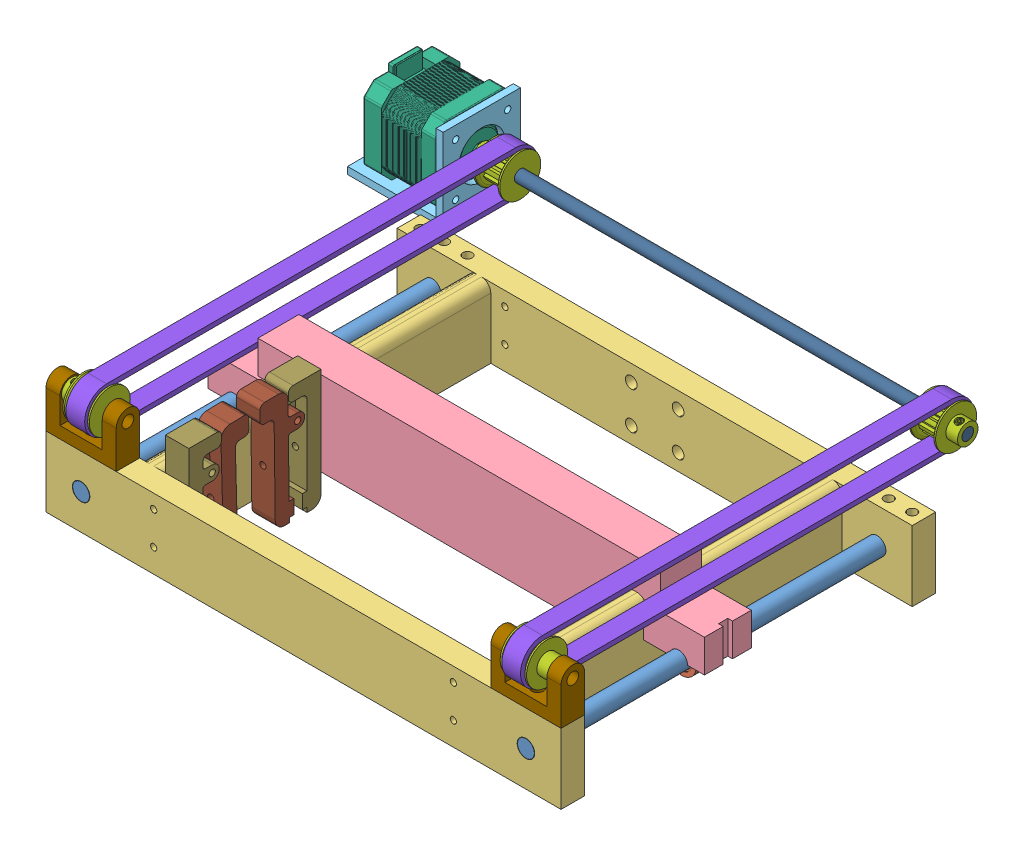
SolidWorks assembly Gantry Assembly Vertical Pulleys, configuration Default. Lengths in mm.
Overall size (322.83 91.67 256.35).
24 component instances, 12 part files, 42 mates.
Components (placement in the parent):
- 1555T132_Linear Motion Shaft-1: 1555T132_Linear Motion Shaft [1555T132] at (256.3952 90.1087 151.9483) x (0.714788 0.699342 0) z (0 0 1) size (9.53 9.53 203.2)
- 6630K12_Self-Aligning Linear Ball Bearing-1: 6630K12_Self-Aligning Linear Ball Bearing [6630K12] at (256.3952 90.1087 157.9768) size (15.88 15.88 22.23)
- Frame-1: Frame [Default] at (135.7452 70.9617 151.9483) x (0 0 -1) z (1 0 0) size (203.2 38.1 279.4)
- Singular Gantry-1: Singular Gantry [Default] at (135.7452 107.8887 157.9768) size (269.24 45.72 25.4)
- 1555T132_Linear Motion Shaft-2: 1555T132_Linear Motion Shaft [1555T132] at (15.0952 90.1087 151.9483) x (-0.570511 -0.82129 0) z (0 0 -1) size (9.53 9.53 203.2)
- 6630K12_Self-Aligning Linear Ball Bearing-2: 6630K12_Self-Aligning Linear Ball Bearing [6630K12] at (15.0952 90.1087 157.9768) x (0.996009 -0.089256 0) z (0 0 1) size (15.88 15.88 22.23)
- Mount and Motor-1: Mount and Motor [Default] at (-234.8386 169.217 17.6112) x (0 0 -1) z (1 0 0) size (42.51 50.31 70.26)
  - Mount (not Blake)-1: Mount (not Blake) [Default] at (-7.9724 -40.1303 235.4559) x (0 0 1) z (0 1 0) size (51.82 41.92 45.73)
  - Stepper Motor-1: Stepper Motor [Default] at (-7.6774 -39.8353 216.7059) size (42.5 46.5 61.75)
- 6495K744_Timing Belt Pulley-9: 6495K744_Timing Belt Pulley [6495K744] at (14.7396 129.3817 25.2886) x (0 -0.489559 0.87197) z (-1 0 0) size (22.23 22.23 20.62)
- Linear Rod Belt-1: Linear Rod Belt [Default] at (259.0495 129.3817 136.2434) x (0 0 -1) z (0 1 0) size (245.79 10.16 23.88)
- Linear Rod Belt-2: Linear Rod Belt [Default] at (12.4409 129.3817 136.2434) x (0 0 -1) z (0 -1 0) size (245.79 10.16 23.88)
- 6495K744_Timing Belt Pulley-10: 6495K744_Timing Belt Pulley [6495K744] at (13.9776 129.3817 247.1983) x (0 0.986803 0.161926) z (-1 0 0) size (22.23 22.23 20.62)
- Sideways Pulley Holder-1: Sideways Pulley Holder [Default] at (-3.9548 109.0617 247.1983) size (38.1 26.67 12.7)
- Sideways Pulley Holder-2: Sideways Pulley Holder [Default] at (237.3452 109.0617 247.1983) size (38.1 26.67 12.7)
- 6495K744_Timing Belt Pulley-11: 6495K744_Timing Belt Pulley [6495K744] at (257.5128 129.3817 247.1983) x (0 -0.977894 -0.209101) z (1 0 0) size (22.23 22.23 20.62)
- 6495K744_Timing Belt Pulley-12: 6495K744_Timing Belt Pulley [6495K744] at (257.5128 129.3817 25.2886) x (0 0.264564 -0.964368) z (1 0 0) size (22.23 22.23 20.62)
- Sideways Pulley Long Axle-1: Sideways Pulley Long Axle [Default] at (267.8252 129.3817 25.2886) x (0 -0.963895 0.266284) z (0 -0.266284 -0.963895) size (6.35 254 6.35)
- Clip Assembly-3: Clip Assembly [Default] at (102.1447 55.2873 173.3888) x (0 0.02134 0.999772) z (-1 0 0) size (34.59 64.43 12.7) (flexible)
  - Added Clip Piece-1: Added Clip Piece [Default] at (17.9829 40.6841 41.3294) x (0.999416 -0.034157 0) z (0 0 1) size (24.13 63.5 12.7)
  - Attatched Clip Piece-1: Attatched Clip Piece [Default] at (0.3891 41.1725 54.0294) x (-0.999772 0.02134 0) z (0 0 -1) size (17.78 63.5 12.7)
- Clip Assembly-5: Clip Assembly [Default] at (6.7858 53.9203 236.5487) x (0 0.02134 -0.999772) z (1 0 0) size (34.27 63.86 12.7) (flexible)
  - Added Clip Piece-1: Added Clip Piece [Default] at (18.5505 41.0342 41.3294) x (0.999981 0.006111 0) z (0 0 1) size (24.13 63.5 12.7)
  - Attatched Clip Piece-1: Attatched Clip Piece [Default] at (0.3891 41.1725 54.0294) x (-0.999772 0.02134 0) z (0 0 -1) size (17.78 63.5 12.7)
Mates (geometry in assembly coordinates):
- Concentric1: concentric anti-aligned: cylinder of 6630K12_Self-Aligning Linear Ball Bearing-1 through (256.3952 90.1087 169.0893) axis (0 0 -1) radius 7.9375; cylinder of Singular Gantry-1 through (256.3952 90.1087 146.8643) axis (0 0 1) radius 7.9375
- Coincident1: coincident anti-aligned: plane of 6630K12_Self-Aligning Linear Ball Bearing-1 through (256.3952 90.1087 146.8643) normal (0 0 -1); plane of Singular Gantry-1 through (15.0952 90.1087 146.8643) normal (0 0 1)
- Concentric2: concentric aligned: cylinder of 1555T132_Linear Motion Shaft-1 through (256.3952 90.1087 253.5483) axis (0 0 -1) radius 4.7625; cylinder of 6630K12_Self-Aligning Linear Ball Bearing-1 through (256.3952 90.1087 169.0893) axis (0 0 -1) radius 4.8895
- Concentric3: concentric anti-aligned: cylinder of 1555T132_Linear Motion Shaft-1 through (256.3952 90.1087 253.5483) axis (0 0 -1) radius 4.7625; cylinder of Frame-1 through (256.3952 90.1087 -189.6817) axis (0 0 1) radius 4.7625
- Concentric4: concentric aligned: cylinder of Frame-1 through (15.0952 90.1087 -189.6817) axis (0 0 1) radius 4.7625; cylinder of 1555T132_Linear Motion Shaft-2 through (15.0952 90.1087 50.3483) axis (0 0 1) radius 4.7625
- Parallel1: parallel aligned: plane of Frame-1 through (135.7452 109.0617 151.9483) normal (0 1 0); plane of Singular Gantry-1 through (26.5252 125.6687 146.8643) normal (0 1 0)
- Concentric5: concentric anti-aligned: cylinder of Singular Gantry-1 through (15.0952 90.1087 146.8643) axis (0 0 1) radius 7.9375; cylinder of 6630K12_Self-Aligning Linear Ball Bearing-2 through (15.0952 90.1087 169.0893) axis (0 0 -1) radius 7.9375
- Coincident2: coincident anti-aligned: plane of Singular Gantry-1 through (15.0952 90.1087 146.8643) normal (0 0 1); plane of 6630K12_Self-Aligning Linear Ball Bearing-2 through (15.0952 90.1087 146.8643) normal (0 0 -1)
- Concentric6: concentric anti-aligned: cylinder of 1555T132_Linear Motion Shaft-2 through (15.0952 90.1087 50.3483) axis (0 0 1) radius 4.7625; cylinder of 6630K12_Self-Aligning Linear Ball Bearing-2 through (15.0952 90.1087 169.0893) axis (0 0 -1) radius 4.8895
- Coincident3: coincident aligned: plane of Frame-1 through (275.4452 109.0617 253.5483) normal (0 0 1); circle of 1555T132_Linear Motion Shaft-2
- Coincident4: coincident aligned: plane of 1555T132_Linear Motion Shaft-1 through (256.3952 90.1087 253.5483) normal (0 0 1); plane of Frame-1 through (275.4452 109.0617 253.5483) normal (0 0 1)
- Concentric18: concentric aligned: cylinder of Mount and Motor-1/Stepper Motor-1 through (22.8672 129.3817 25.2886) axis (-1 0 0) radius 2.5; cylinder of 6495K744_Timing Belt Pulley-9 through (4.4272 129.3817 25.2886) axis (-1 0 0) radius 3.175
- Coincident13: coincident anti-aligned: plane of Mount and Motor-1/Mount (not Blake)-1 through (4.4272 129.0867 25.5836) normal (1 0 0); plane of 6495K744_Timing Belt Pulley-9 through (4.4272 126.6132 23.7343) normal (-1 0 0)
- Concentric21: concentric anti-aligned: cylinder of Frame-1 through (15.0952 109.0617 247.1983) axis (0 -1 0) radius 2.54; cylinder of Sideways Pulley Holder-1 through (15.0952 90.0117 247.1983) axis (0 1 0) radius 3.175
- Coincident31: coincident aligned: plane of Frame-1 through (275.4452 109.0617 253.5483) normal (0 0 1); plane of Sideways Pulley Holder-1 through (34.1452 109.0617 253.5483) normal (0 0 1)
- Coincident32: coincident anti-aligned: plane of Frame-1 through (135.7452 109.0617 151.9483) normal (0 1 0); plane of Sideways Pulley Holder-1 through (34.1452 109.0617 253.5483) normal (0 -1 0)
- Concentric22: concentric aligned: cylinder of 6495K744_Timing Belt Pulley-10 through (3.6652 129.3817 247.1983) axis (-1 0 0) radius 3.175; cylinder of Sideways Pulley Holder-1 through (34.1452 129.3817 247.1983) axis (-1 0 0) radius 3.175
- Coincident33: coincident anti-aligned: plane of 6495K744_Timing Belt Pulley-10 through (3.6652 128.8676 250.3314) normal (-1 0 0); plane of Sideways Pulley Holder-1 through (3.6652 135.7317 228.1483) normal (1 0 0)
- Concentric23: concentric anti-aligned: circle of Linear Rod Belt-2; circle of 6495K744_Timing Belt Pulley-10
- Coincident34: coincident anti-aligned: plane of Linear Rod Belt-2 through (22.6009 129.3817 247.1983) normal (1 0 0); plane of 6495K744_Timing Belt Pulley-10 through (22.6009 128.1128 254.9307) normal (-1 0 0)
- Concentric24: concentric anti-aligned: circle of 6495K744_Timing Belt Pulley-9; circle of Linear Rod Belt-2
- Coincident35: coincident anti-aligned: plane of 6495K744_Timing Belt Pulley-9 through (12.4409 121.1205 20.6504) normal (1 0 0); plane of Linear Rod Belt-2 through (12.4409 129.3817 247.1983) normal (-1 0 0)
- Parallel6: parallel anti-aligned: plane of Frame-1 through (135.7452 109.0617 151.9483) normal (0 1 0); plane of Mount and Motor-1/Mount (not Blake)-1 through (0.6172 104.3217 25.5836) normal (0 -1 0)
- Parallel7: parallel aligned: plane of Frame-1 through (135.7452 109.0617 151.9483) normal (0 1 0); plane of Linear Rod Belt-2 through (22.6009 141.3197 247.1983) normal (0 1 0)
- Concentric25: concentric anti-aligned: cylinder of Frame-1 through (256.3952 109.0617 247.1983) axis (0 -1 0) radius 2.54; cylinder of Sideways Pulley Holder-2 through (256.3952 90.0117 247.1983) axis (0 1 0) radius 3.175
- Coincident38: coincident aligned: plane of Frame-1 through (275.4452 109.0617 253.5483) normal (0 0 1); plane of Sideways Pulley Holder-2 through (275.4452 109.0617 253.5483) normal (0 0 1)
- Coincident39: coincident anti-aligned: plane of Frame-1 through (135.7452 109.0617 151.9483) normal (0 1 0); plane of Sideways Pulley Holder-2 through (275.4452 109.0617 253.5483) normal (0 -1 0)
- Concentric26: concentric anti-aligned: cylinder of Sideways Pulley Holder-2 through (275.4452 129.3817 247.1983) axis (-1 0 0) radius 3.175; cylinder of 6495K744_Timing Belt Pulley-11 through (267.8252 129.3817 247.1983) axis (1 0 0) radius 3.175
- Coincident44: coincident anti-aligned: plane of Sideways Pulley Holder-2 through (267.8252 135.7317 228.1483) normal (-1 0 0); plane of 6495K744_Timing Belt Pulley-11 through (267.8252 128.7178 250.3031) normal (1 0 0)
- Concentric27: concentric anti-aligned: circle of Linear Rod Belt-1; circle of 6495K744_Timing Belt Pulley-11
- Coincident45: coincident anti-aligned: plane of Linear Rod Belt-1 through (248.8895 129.3817 247.1983) normal (-1 0 0); plane of 6495K744_Timing Belt Pulley-11 through (248.8895 127.7432 254.8609) normal (1 0 0)
- Concentric28: concentric anti-aligned: circle of Linear Rod Belt-1; circle of 6495K744_Timing Belt Pulley-12
- Coincident46: coincident anti-aligned: plane of Linear Rod Belt-1 through (248.8895 129.3817 247.1983) normal (-1 0 0); plane of 6495K744_Timing Belt Pulley-12 through (248.8895 121.825 23.2155) normal (1 0 0)
- Concentric29: concentric anti-aligned: cylinder of 6495K744_Timing Belt Pulley-9 through (4.4272 129.3817 25.2886) axis (-1 0 0) radius 3.175; cylinder of Sideways Pulley Long Axle-1 through (13.8252 129.3817 25.2886) axis (1 0 0) radius 3.175
- Concentric30: concentric aligned: cylinder of 6495K744_Timing Belt Pulley-12 through (267.8252 129.3817 25.2886) axis (1 0 0) radius 3.175; cylinder of Sideways Pulley Long Axle-1 through (13.8252 129.3817 25.2886) axis (1 0 0) radius 3.175
- Coincident47: coincident aligned: plane of 6495K744_Timing Belt Pulley-12 through (267.8252 126.3198 24.4486) normal (1 0 0); plane of Sideways Pulley Long Axle-1 through (267.8252 129.3817 25.2886) normal (1 0 0)
- Coincident50: coincident anti-aligned: plane of Singular Gantry-1 through (256.3952 90.1087 169.0893) normal (0 0 1); plane of Clip Assembly-3/Attatched Clip Piece-1 through (60.8152 128.2087 169.0893) normal (0 0 -1)
- Parallel14: parallel anti-aligned: plane of Frame-1 through (46.8452 109.0617 240.8483) normal (1 0 0); plane of Clip Assembly-3/Attatched Clip Piece-1 through (48.1152 69.7887 174.1693) normal (-1 0 0)
- Concentric34: concentric aligned: cylinder of Clip Assembly-3/Attatched Clip Piece-1 through (54.4652 102.8087 156.3893) axis (0 0 1) radius 1.7; cylinder of Singular Gantry-1 through (54.4652 102.8087 146.8643) axis (0 0 1) radius 1.7
- Concentric35: concentric anti-aligned: cylinder of Frame-1 through (54.4652 101.4417 -189.6817) axis (0 0 1) radius 1.7; cylinder of Clip Assembly-5/Attatched Clip Piece-1 through (54.4652 101.4417 253.5483) axis (0 0 -1) radius 1.7
- Coincident51: coincident anti-aligned: plane of Frame-1 through (46.8452 109.0617 240.8483) normal (0 0 -1); plane of Clip Assembly-5/Attatched Clip Piece-1 through (48.1152 126.8417 240.8483) normal (0 0 1)
- Parallel15: parallel anti-aligned: plane of Frame-1 through (46.8452 109.0617 240.8483) normal (1 0 0); plane of Clip Assembly-5/Added Clip Piece-1 through (48.1152 68.6462 219.4156) normal (-1 0 0)
